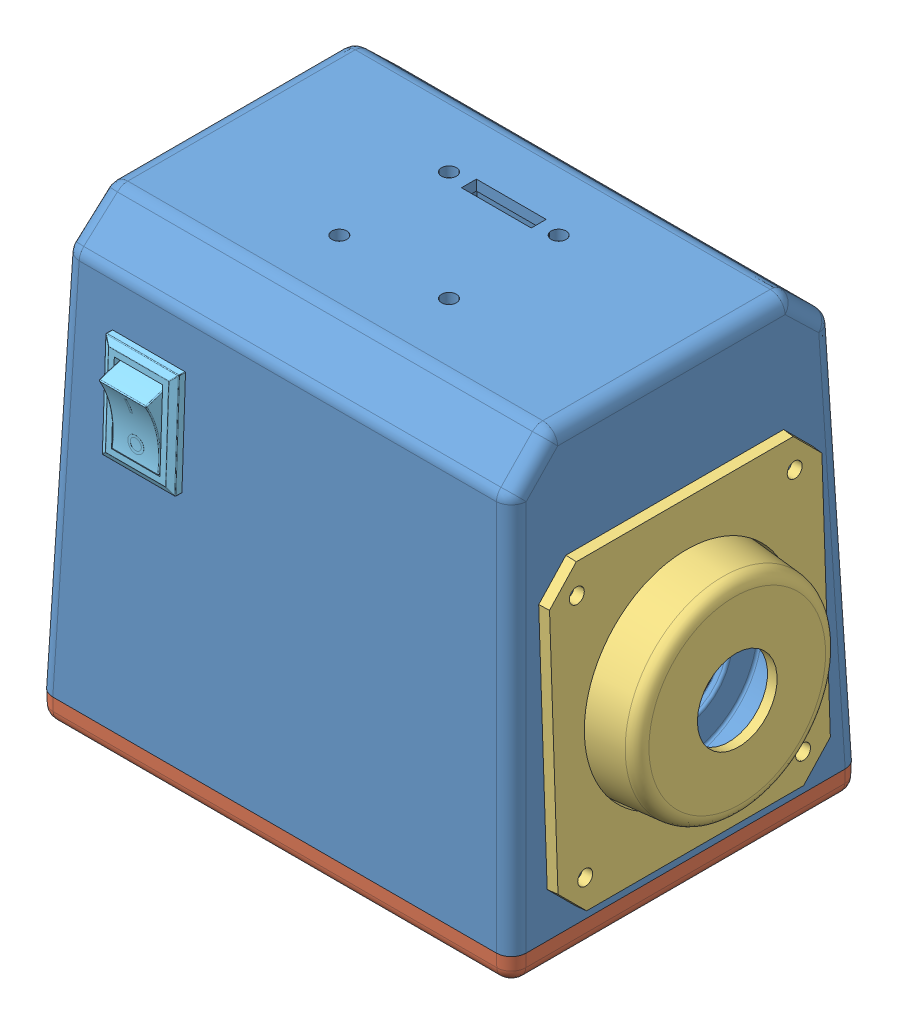
SolidWorks assembly Assem1, configuration Default. Lengths in mm.
Overall size (118.95 90 73.68).
6 component instances, 5 part files, 2 mates.
Components (placement in the parent):
- Top_Part-1: Top_Part [Default] at origin size (113.85 85 70)
- Bottom_Part-1: Bottom_Part [Default] at origin size (95.34 5 70.34)
- Side_Part-1: Side_Part [Default] at origin size (15.05 59.96 55)
- Side_Part-2: Side_Part [Default] x (-1 0 0) z (0 0 -1) size (15.05 59.96 55)
- PCB2.step-1: PCB2.step [Default] at (-20 65 -22.5) x (1 0 0) z (0 -1 0) size (60.8 44.93 12.39)
- switch-1: switch [Default] at (-27.5785 57.0885 33.0064) x (0 -0.999391 0.034899) z (0 0.034899 0.999391) size (21.1 14.71 23.64)
Mates (geometry in assembly coordinates):
- Parallel2: parallel anti-aligned: plane of Top_Part-1 through (0 83 0) normal (0 -1 0); plane of PCB2.step-1 through (10.4783 66.2 -0.1226) normal (0 1 0)
- Coincident3: coincident anti-aligned: plane of Top_Part-1 through (-47.5 0 35) normal (0 0.034899 0.999391); plane of switch-1 through (-27.5785 57.0885 33.0064) normal (0 -0.034899 -0.999391)
